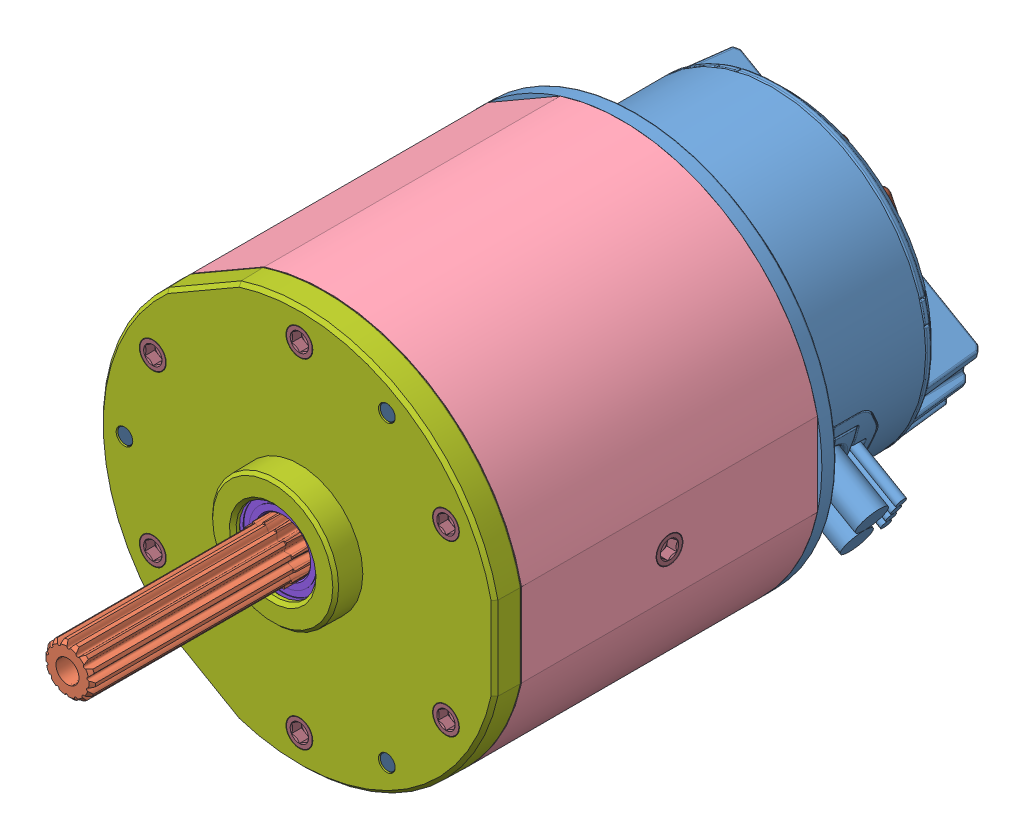
SolidWorks assembly Falcon_500_Powered_by_Talon_FX_217-6515, configuration Default. Lengths in mm.
Overall size (81.66 81.44 116.05).
29 component instances, 13 part files, 0 mates.
Components (placement in the parent):
- 217-6515-Back 20190920-1: 217-6515-Back 20190920 [Default] at (1.2326 6.2358 -14.9619) size (60 60 78.85)
- 217-6515-200 Rev5-1: 217-6515-200 Rev5 [Default] at (1.2326 6.2358 29.5381) x (0.809017 0.587785 0) z (0 0 1) size (20 20 42.2)
  - 217-6515-201 Rev6-1: 217-6515-201 Rev6 [Default] at (0 0 21.1) size (9.31 9.33 42.2)
  - 217-6515-202 Rev6-1: 217-6515-202 Rev6 [Default] x (-1 0 0) z (0 1 0) size (20 5.23 20)
- 217-6515-002 Rev6-1: 217-6515-002 Rev6 [Default] at (1.2326 6.2358 10.7381) x (0 -1 0) z (0 0 1) size (60 59.34 44.4)
- M2.5 SHCS, Grade 8 Steel Rev1_SSAM2.5-06MMZB-1: M2.5 SHCS, Grade 8 Steel Rev1_SSAM2.5-06MMZB [Default] at (-5.4248 8.3989 26.0381) x (-0.940162 0.340727 0) z (0 0 -1) size (4.5 4.5 8.62)
- M2.5 SHCS, Grade 8 Steel Rev1_SSAM2.5-06MMZB-2: M2.5 SHCS, Grade 8 Steel Rev1_SSAM2.5-06MMZB [Default] at (1.2326 13.2358 26.0381) x (0.033525 0.999438 0) z (0 0 -1) size (4.5 4.5 8.62)
- M2.5 SHCS, Grade 8 Steel Rev1_SSAM2.5-06MMZB-3: M2.5 SHCS, Grade 8 Steel Rev1_SSAM2.5-06MMZB [Default] at (7.89 8.3989 26.0381) x (0.960882 0.27696 0) z (0 0 -1) size (4.5 4.5 8.62)
- M2.5 SHCS, Grade 8 Steel Rev1_SSAM2.5-06MMZB-4: M2.5 SHCS, Grade 8 Steel Rev1_SSAM2.5-06MMZB [Default] at (5.3471 0.5727 26.0381) x (0.560333 -0.828267 0) z (0 0 -1) size (4.5 4.5 8.62)
- M2.5 SHCS, Grade 8 Steel Rev1_SSAM2.5-06MMZB-5: M2.5 SHCS, Grade 8 Steel Rev1_SSAM2.5-06MMZB [Default] at (-2.8819 0.5727 26.0381) x (-0.614577 -0.788857 0) z (0 0 -1) size (4.5 4.5 8.62)
- 217-6515-010 Rev1_9262K442-1: 217-6515-010 Rev1_9262K442 [Default] at (1.2326 6.2358 35.0381) size (10 10 1)
- 217-6515-001 Rev6-1: 217-6515-001 Rev6 [Default] at (1.2326 6.2358 30.9381) x (0.5 0.866025 0) z (0 0 1) size (59.4 60 10)
- 217-6515-005 Rev4_7804K116-1: 217-6515-005 Rev4_7804K116 [Default] at (1.2326 6.2358 37.4381) size (14 14 4)
- M3 BHTS-SECURE, Grade 8 Steel Rev1_SBTM3-24MMZB-SECURE-1: M3 BHTS-SECURE, Grade 8 Steel Rev1_SBTM3-24MMZB-SECURE [Default] at (9.7324 20.9581 -38.0119) x (-0.923728 -0.383049 0) z (0 0 -1) size (5.73 5.74 26.03)
- M3 BHTS-SECURE, Grade 8 Steel Rev1_SBTM3-24MMZB-SECURE-2: M3 BHTS-SECURE, Grade 8 Steel Rev1_SBTM3-24MMZB-SECURE [Default] at (-15.7672 6.2357 -38.0119) x (0.793594 -0.608447 0) z (0 0 -1) size (5.73 5.74 26.03)
- M3 BHTS-SECURE, Grade 8 Steel Rev1_SBTM3-24MMZB-SECURE-3: M3 BHTS-SECURE, Grade 8 Steel Rev1_SBTM3-24MMZB-SECURE [Default] at (9.7326 -8.4864 -38.0119) x (0.130134 0.991496 0) z (0 0 -1) size (5.73 5.74 26.03)
- M3 BHTS, Grade 8 Steel Rev1_SBTM3-50MMZB-1: M3 BHTS, Grade 8 Steel Rev1_SBTM3-50MMZB [Default] at (14.3576 28.969 -14.8619) x (-0.923728 -0.383049 0) z (0 0 -1) size (5.74 5.77 52.03)
- M3 BHTS, Grade 8 Steel Rev1_SBTM3-50MMZB-2: M3 BHTS, Grade 8 Steel Rev1_SBTM3-50MMZB [Default] at (-25.0174 6.2358 -14.8619) x (0.793594 -0.608447 0) z (0 0 -1) size (5.74 5.77 52.03)
- M3 BHTS, Grade 8 Steel Rev1_SBTM3-50MMZB-3: M3 BHTS, Grade 8 Steel Rev1_SBTM3-50MMZB [Default] at (14.3576 -16.4974 -14.8619) x (0.130134 0.991496 0) z (0 0 -1) size (5.74 5.77 52.03)
- 217-6515-308 Rev5-1: 217-6515-308 Rev5 [Default] at (7.0724 16.3512 -38.3619) x (0.866013 -0.500022 0) z (0.500022 0.866013 0) size (21.32 4.26 9.98)
- #4-40 SHCS, Grade 8 Steel Rev2_SSA0440-0125ZB-1: #4-40 SHCS, Grade 8 Steel Rev2_SSA0440-0125ZB [Default] at (-1.3722 18.2247 -35.6869) x (-0.90374 0.428082 0) z (0 0 -1) size (4.65 4.65 6.16)
- #4-40 SHCS, Grade 8 Steel Rev2_SSA0440-0125ZB-2: #4-40 SHCS, Grade 8 Steel Rev2_SSA0440-0125ZB [Default] at (12.917 9.9744 -35.6869) x (-0.992189 0.124742 0) z (0 0 -1) size (4.65 4.65 6.16)
- 217-4649-007 Rev1_94105A824_1-1: 217-4649-007 Rev1_94105A824_1 [Default] at (1.2326 31.6358 34.9541) size (4.83 4.83 4.9)
- 217-4649-007 Rev1_94105A824_1-2: 217-4649-007 Rev1_94105A824_1 [Default] at (28.5903 6.2358 10.7381) x (0 -0.924225 -0.381849) z (1 0 0) size (4.83 4.83 4.9)
- 217-4649-007 Rev1_94105A824_1-3: 217-4649-007 Rev1_94105A824_1 [Default] at (23.2296 18.9358 34.9541) x (0.5 -0.866025 0) z (0 0 1) size (4.83 4.83 4.9)
- 217-4649-007 Rev1_94105A824_1-4: 217-4649-007 Rev1_94105A824_1 [Default] at (23.2296 -6.4642 34.9541) x (-0.5 -0.866025 0) z (0 0 1) size (4.83 4.83 4.9)
- 217-4649-007 Rev1_94105A824_1-5: 217-4649-007 Rev1_94105A824_1 [Default] at (1.2326 -19.1642 34.9541) x (-1 0 0) z (0 0 1) size (4.83 4.83 4.9)
- 217-4649-007 Rev1_94105A824_1-6: 217-4649-007 Rev1_94105A824_1 [Default] at (-20.7645 -6.4642 34.9541) x (-0.5 0.866025 0) z (0 0 1) size (4.83 4.83 4.9)
- 217-4649-007 Rev1_94105A824_1-7: 217-4649-007 Rev1_94105A824_1 [Default] at (-20.7645 18.9358 34.9541) x (0.5 0.866025 0) z (0 0 1) size (4.83 4.83 4.9)
